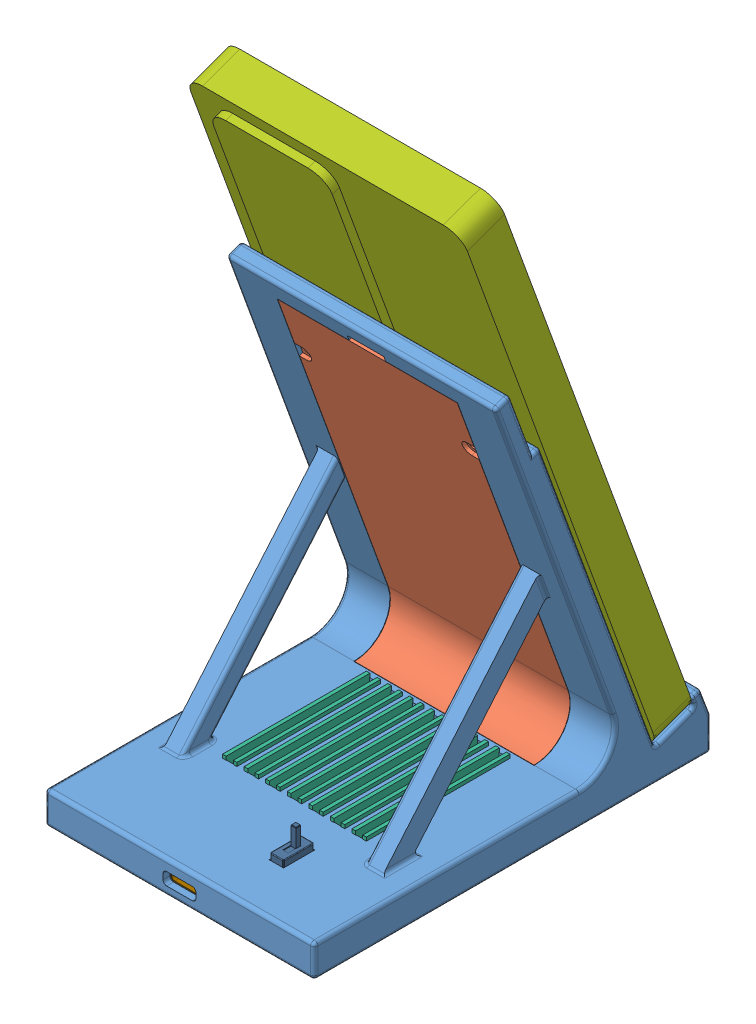
SolidWorks assembly IP支架装配体, configuration 默认. Lengths in mm.
Overall size (77 164.05 111.5).
31 component instances, 16 part files, 23 mates.
Components (placement in the parent):
- IP支架-1: IP支架 [默认] at (-19.3867 -35.6954 110) size (75 113.62 110.5)
- 支架零件-1: 支架零件 [默认] at (-19.3867 -31.7451 120.1792) x (0 0 -1) z (1 0 0) size (34.38 102 50)
- IP手机-1: IP手机 [默认] at (-19.3867 44.2514 95.8225) x (1 0 0) z (0 0.939693 0.34202) size (76 12 151) (hidden)
- 充电线圈-1: 充电线圈 [默认] at (-19.3867 48.3322 101.4581) x (1 0 0) z (0 -0.939693 -0.34202) size (43 1.52 55.03)
- 充电零件板-1: 充电零件板 [默认] at (-19.3867 -30.6954 114.2678) x (1 0 0) z (0 0 -1) size (21 2 28)
- 底板-1: 底板 [默认] at (-34.8284 -35.6954 107.1856) x (0 0 -1) z (1 0 0) size (101.9 5.8 64.8)
- 散热器-1: 散热器 [默认] at (-19.3867 -30.6954 113) size (40 5 40)
- P60手机-1: P60手机 [默认] at (-19.3867 48.9499 97.5326) x (-1 0 0) z (0 0.34202 -0.939693) size (77 161 13.1)
- TypeC电路板-2: TypeC电路板 [默认] at (-41.3838 -28.6954 166.3115) x (0 0 -1) z (0 -1 0) size (30 34.97 13.16)
  - TypeC电路板.STEP-1: TypeC电路板.STEP [默认] at origin size (30 34.97 13.16)
    - TypeC______.STEP.STEP-1: TypeC______.STEP.STEP [默认] at origin size (30 34.97 13.16)
      - 5v06-R1.STEP.STEP-1: 5v06-R1.STEP.STEP [默认] at (25.0953 30.8357 1.2) x (-1 0 0) z (0 0 1) size (2 1.3 0.61)
        - R0805.STEP.STEP-1: R0805.STEP.STEP [默认] at origin size (2 1.3 0.61)
          - COMPOUND.STEP.STEP-1: COMPOUND.STEP.STEP [默认] at origin size (2 1.3 0.61)
      - 5v06-USB1.STEP.STEP-1: 5v06-USB1.STEP.STEP [默认] at (8.1992 21.9972 1.2) x (0 -1 0) z (0 0 1) size (8.95 7.58 4.16)
        - USB-C-SMD_TYPE-C-6PIN-2MD-073.STEP.STEP-1: USB-C-SMD_TYPE-C-6PIN-2MD-073.STEP.STEP [默认] at origin size (8.95 7.58 4.16)
          - COMPOUND-1.STEP.STEP-1: COMPOUND-1.STEP.STEP [默认] at origin size (8.95 7.58 4.16)
      - 5v06-U2.STEP.STEP-1: 5v06-U2.STEP.STEP [默认] at (19.685 34.9251 0) x (-1 0 0) z (0 0 -1) size (8.51 3.81 11.5)
        - SW-TH_DEALON_SS-12D01-GX.STEP.STEP-1: SW-TH_DEALON_SS-12D01-GX.STEP.STEP [默认] at origin size (8.51 3.81 11.5)
          - COMPOUND-2.STEP.STEP-1: COMPOUND-2.STEP.STEP [默认] at origin size (8.51 3.81 11.5)
      - 5v06-C1.STEP.STEP-1: 5v06-C1.STEP.STEP [默认] at (18.2118 28.8799 1.2) size (3.2 2.52 0.9)
        - C1210.STEP.STEP-1: C1210.STEP.STEP [默认] at origin size (3.2 2.52 0.9)
          - SOLID-3.STEP.STEP-1: SOLID-3.STEP.STEP [默认] at origin size (3.2 2.52 0.9)
      - 5v06-C2.STEP.STEP-1: 5v06-C2.STEP.STEP [默认] at (24.13 13.843 1.2) x (0 1 0) z (0 0 1) size (1.6 0.8 0.8)
        - C0603.STEP.STEP-1: C0603.STEP.STEP [默认] at origin size (1.6 0.8 0.8)
          - SOLID-4.STEP.STEP-1: SOLID-4.STEP.STEP [默认] at origin size (1.6 0.8 0.8)
      - 5v06-U4.STEP.STEP-1: 5v06-U4.STEP.STEP [默认] at (18.386 14.645 1.2) size (4.1 4.3 1.61)
        - SOT-89-3_L4.5-W2.5-P1.50-LS4.2-BR.STEP.STEP-1: SOT-89-3_L4.5-W2.5-P1.50-LS4.2-BR.STEP.STEP [默认] at origin size (4.1 4.3 1.61)
          - SOLID-5.STEP.STEP-1: SOLID-5.STEP.STEP [默认] at origin size (4.1 4.3 1.61)
      - Board.STEP.STEP-1: Board.STEP.STEP [默认] at origin size (29.97 34.97 1.2)
- Led5mmRojo_.step-1: Led5mmRojo_.step [默认] at (-19.3867 -31.1954 79) x (0 0 -1) z (1 0 0) size (25.5 5.8 5.4)
Mates (geometry in assembly coordinates):
- 重合1: coincident anti-aligned: plane of IP支架-1 through (132.7849 78.9281 108.4438) normal (0 0.34202 -0.939693); plane of IP手机-1 through (-19.3867 44.2514 95.8225) normal (0 -0.34202 0.939693)
- 宽度1: width aligned: plane of IP支架-1 through (18.1133 -26.6954 165) normal (1 0 0); plane of IP手机-1 through (-56.8867 -26.6954 165) normal (-1 0 0); plane of IP支架-1 through (18.6133 -22.9332 59.6634) normal (1 0 0); plane of IP手机-1 through (-57.3867 -22.9332 59.6634) normal (-1 0 0)
- 重合8: coincident anti-aligned: plane of 支架零件-1 through (-19.3867 47.8192 102.8677) normal (0 0.34202 -0.939693); plane of 充电线圈-1 through (-19.3867 47.8192 102.8677) normal (0 -0.34202 0.939693)
- 同心1: concentric aligned: cylinder of 支架零件-1 through (-19.3867 47.8192 102.8677) axis (0 0.34202 -0.939693) radius 22; cylinder of 充电线圈-1 through (-19.3867 47.8192 102.8677) axis (0 0.34202 -0.939693) radius 21.5
- 重合15: coincident aligned: plane of 支架零件-1 through (-19.3867 -31.7451 120.1792) normal (1 0 0); plane of 充电线圈-1 through (-19.3867 48.3322 101.4581) normal (1 0 0)
- 宽度8: width aligned: plane of IP支架-1 through (18.1133 -26.6954 165) normal (1 0 0); plane of IP支架-1 through (-56.8867 -26.6954 165) normal (-1 0 0); plane of 散热器-1 through (0.6133 -28.6954 93) normal (1 0 0); plane of 散热器-1 through (-39.3867 -28.6954 93) normal (-1 0 0)
- 距离4: distance = 32 mm aligned: plane of 散热器-1 through (-39.3867 -28.6954 133) normal (0 0 1); plane of IP支架-1 through (-56.8867 -26.6954 165) normal (0 0 1)
- 重合43: coincident anti-aligned: plane of 充电零件板-1 through (-21.3867 -30.6954 108.6428) normal (0 1 0); plane of 散热器-1 through (-19.3867 -30.6954 113) normal (0 -1 0)
- 宽度9: width aligned: plane of 散热器-1 through (-39.3867 -28.6954 93) normal (-1 0 0); plane of 充电零件板-1 through (0.6133 -28.6954 93) normal (1 0 0); plane of 散热器-1 through (-29.8867 -32.6954 125.2678) normal (-1 0 0); plane of 充电零件板-1 through (-8.8867 -32.6954 125.2678) normal (1 0 0)
- 重合44: coincident aligned: plane of IP支架-1 through (-19.3867 -35.6954 110) normal (0 -1 0); plane of 底板-1 through (-34.8284 -35.6954 107.1856) normal (0 -1 0)
- 宽度11: width anti-aligned: plane of IP支架-1 through (-400019.3867 -35.6964 159) normal (0 0 -1); plane of IP支架-1 through (-400019.3867 -35.6964 61) normal (0 0 1); plane of 底板-1 through (-51.7867 -34.1954 158.9) normal (0 0 1); plane of 底板-1 through (-51.7867 -34.1954 61.1) normal (0 0 -1)
- 重合50: coincident anti-aligned: plane of IP支架-1 through (132.7849 78.9281 108.4438) normal (0 0.34202 -0.939693); plane of P60手机-1 through (-19.3867 48.9499 97.5326) normal (0 -0.34202 0.939693)
- 重合51: coincident anti-aligned: plane of IP支架-1 through (-79.7288 -26.6954 70) normal (0 0.939693 0.34202); plane of P60手机-1 through (19.1133 -22.9332 59.6634) normal (0 -0.939693 -0.34202)
- 宽度14: width aligned: plane of P60手机-1 through (19.1133 128.3573 114.7286) normal (1 0 0); plane of P60手机-1 through (-57.8867 128.3573 114.7286) normal (-1 0 0); plane of IP支架-1 through (18.1133 -26.6954 165) normal (1 0 0); plane of IP支架-1 through (-56.8867 -26.6954 165) normal (-1 0 0)
- 重合52: coincident anti-aligned: plane of IP支架-1 through (-79.7288 -26.6954 70) normal (0 0.939693 0.34202); plane of IP手机-1 through (-57.3867 -22.9332 59.6634) normal (0 -0.939693 -0.34202)
- 距离9: distance = 0.1 mm anti-aligned: plane of TypeC电路板-2/TypeC电路板.STEP-1/TypeC______.STEP.STEP-1/Board.STEP.STEP-1 through (-1.8994 -28.6954 133.1) normal (0 0 -1); plane of 散热器-1 through (-39.3867 -28.6954 133) normal (0 0 1)
- 宽度15: width aligned: plane of IP支架-1 through (13.1133 -35.6964 291654.25) normal (-1 0 0); plane of TypeC电路板-2/TypeC电路板.STEP-1/TypeC______.STEP.STEP-1/Board.STEP.STEP-1 through (-51.8867 -35.6964 291654.25) normal (1 0 0); plane of IP支架-1 through (-36.874 -28.6954 133.1) normal (-1 0 0); plane of TypeC电路板-2/TypeC电路板.STEP-1/TypeC______.STEP.STEP-1/Board.STEP.STEP-1 through (-1.8994 -28.6954 155.5746) normal (1 0 0)
- 宽度16: width: plane of IP支架-1 through (-19.3867 -35.6954 110) normal (0 -1 0); plane of IP支架-1 through (-19.3867 -26.6954 110) normal (0 1 0); cylinder of Led5mmRojo_.step-1 through (-19.3867 -31.1954 61) axis (0 0 -1) radius 2.5
- 宽度17: width: plane of IP支架-1 through (18.1133 -26.6954 165) normal (1 0 0); plane of IP支架-1 through (-56.8867 -26.6954 165) normal (-1 0 0); cylinder of Led5mmRojo_.step-1 through (-19.3867 -31.1954 61) axis (0 0 -1) radius 2.5
- 平行1: parallel aligned: plane of IP支架-1 through (-19.3867 -35.6954 110) normal (0 -1 0); plane of Led5mmRojo_.step-1 through (-18.3667 -31.4454 62) normal (0 -1 0)
- 重合55: coincident anti-aligned: plane of IP支架-1 through (-400019.3867 -35.6964 61) normal (0 0 1); plane of Led5mmRojo_.step-1 through (-19.1867 -31.1954 61) normal (0 0 -1)
- 重合56: coincident anti-aligned: plane of IP支架-1 through (-19.3867 -28.6954 110) normal (0 -1 0); plane of TypeC电路板-2/TypeC电路板.STEP-1/TypeC______.STEP.STEP-1/Board.STEP.STEP-1 through (-19.3867 -28.6954 146.7586) normal (0 1 0)
- 重合57: coincident anti-aligned: plane of IP支架-1 through (-19.3867 -28.6954 110) normal (0 -1 0); plane of 散热器-1 through (-19.3867 -28.6954 113) normal (0 1 0)
